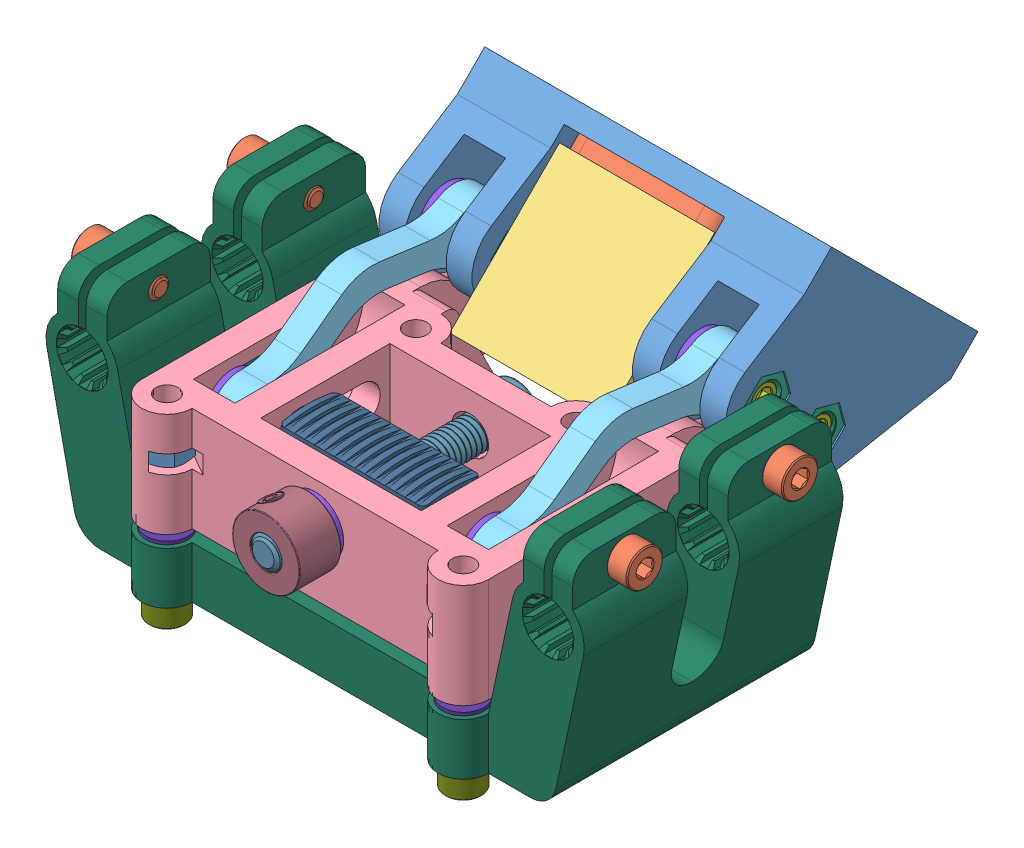
SolidWorks assembly Camera_Angle_Assembly, configuration Default. Lengths in mm.
Overall size (107.85 63.53 108.07).
83 component instances, 20 part files, 71 mates.
Components (placement in the parent):
- Camera_Swing_Bracket-1: Camera_Swing_Bracket [Default] at (-0.7755 -10.5487 -2.6494) x (1 0 0) z (0 -0.707107 0.707107) size (67 43.1 30.6)
- Adapter_Appr-1: Adapter_Appr [Default] at (-30.7755 -11.079 -1.412) x (0 0.707107 0.707107) z (-1 0 0) size (39 2.5 29)
- Camera_Appr-1: Camera_Appr [Default] at (-1.2755 -4.7151 47.3784) x (-1 0 0) z (0 -0.707107 0.707107) size (30 50 30)
- Body_Bracket-2: Body_Bracket [Default] at (-0.7755 -8.7809 23.8671) size (67 20.14 76.95)
- 42-72mm_Linkage_bent_angle-3: 42-72mm_Linkage_bent_angle [Default] at (5.7245 1.8257 34.4737) x (1 0 0) z (0 -0.248282 0.968688) size (5 16.61 54.86)
- 42-72mm_Linkage_bent_angle-4: 42-72mm_Linkage_bent_angle [Default] at (-43.2755 1.8257 34.4737) x (1 0 0) z (0 -0.248282 0.968688) size (5 16.61 54.86)
- Joint_Fastner_Assem-1: Joint_Fastner_Assem [Default] at (21.1511 -8.2693 35.0642) x (0 0.258819 -0.965926) z (0 0.965926 0.258819) size (12.23 18.38 12.23)
  - M6_Shallow_Nuts-1: M6_Shallow_Nuts [90710A038] at (3.1832 5.8266 9.5982) size (10 3.98 11.55)
  - M6_Shallow_Nuts-2: M6_Shallow_Nuts [90710A038] at (3.1832 20.0266 9.5982) size (10 3.98 11.55)
  - Pivot_Bolts-1: Pivot_Bolts [92605A132] at (3.1832 12.6266 9.5982) x (1 0 0) z (0 -1 0) size (6.16 6.24 17.12)
  - Pivot_Washers-1: Pivot_Washers [98689A115] at (3.1832 15.4266 9.5982) x (0.992908 0 0.118882) z (0 1 0) size (11 11 1.5)
  - Pivot_Washers-2: Pivot_Washers [98689A115] at (3.1832 10.4266 9.5982) x (0.997876 0 -0.065141) z (0 -1 0) size (11 11 1.5)
  - Joint_Bushing-1: Joint_Bushing [Default] at (3.1832 10.4266 9.5982) x (0 1 0) z (0 0 1) size (5 7 7)
- Joint_Fastner_Assem-2: Joint_Fastner_Assem [Default] at (21.1511 -14.3398 15.4198) x (0 0.965926 -0.258819) z (0 0.258819 0.965926) size (12.23 18.38 12.23)
  - M6_Shallow_Nuts-1: M6_Shallow_Nuts [90710A038] at (3.1832 5.8266 9.5982) size (10 3.98 11.55)
  - M6_Shallow_Nuts-2: M6_Shallow_Nuts [90710A038] at (3.1832 20.0266 9.5982) size (10 3.98 11.55)
  - Pivot_Bolts-1: Pivot_Bolts [92605A132] at (3.1832 12.6266 9.5982) x (1 0 0) z (0 -1 0) size (6.16 6.24 17.12)
  - Pivot_Washers-1: Pivot_Washers [98689A115] at (3.1832 15.4266 9.5982) x (0.992908 0 0.118882) z (0 1 0) size (11 11 1.5)
  - Pivot_Washers-2: Pivot_Washers [98689A115] at (3.1832 10.4266 9.5982) x (0.997876 0 -0.065141) z (0 -1 0) size (11 11 1.5)
  - Joint_Bushing-1: Joint_Bushing [Default] at (3.1832 10.4266 9.5982) x (0 1 0) z (0 0 1) size (5 7 7)
- Joint_Fastner_Assem-3: Joint_Fastner_Assem [Default] at (-53.7022 0.2569 19.331) x (0 -0.707107 -0.707107) z (0 -0.707107 0.707107) size (12.23 18.38 12.23)
  - M6_Shallow_Nuts-1: M6_Shallow_Nuts [90710A038] at (3.1832 5.8266 9.5982) size (10 3.98 11.55)
  - M6_Shallow_Nuts-2: M6_Shallow_Nuts [90710A038] at (3.1832 20.0266 9.5982) size (10 3.98 11.55)
  - Pivot_Bolts-1: Pivot_Bolts [92605A132] at (3.1832 12.6266 9.5982) x (1 0 0) z (0 -1 0) size (6.16 6.24 17.12)
  - Pivot_Washers-1: Pivot_Washers [98689A115] at (3.1832 15.4266 9.5982) x (0.992908 0 0.118882) z (0 1 0) size (11 11 1.5)
  - Pivot_Washers-2: Pivot_Washers [98689A115] at (3.1832 10.4266 9.5982) x (0.997876 0 -0.065141) z (0 -1 0) size (11 11 1.5)
  - Joint_Bushing-1: Joint_Bushing [Default] at (3.1832 10.4266 9.5982) x (0 1 0) z (0 0 1) size (5 7 7)
- Joint_Fastner_Assem-4: Joint_Fastner_Assem [Default] at (-53.7022 10.8635 29.9376) x (0 -0.707107 -0.707107) z (0 -0.707107 0.707107) size (12.23 18.38 12.23)
  - M6_Shallow_Nuts-1: M6_Shallow_Nuts [90710A038] at (3.1832 5.8266 9.5982) size (10 3.98 11.55)
  - M6_Shallow_Nuts-2: M6_Shallow_Nuts [90710A038] at (3.1832 20.0266 9.5982) size (10 3.98 11.55)
  - Pivot_Bolts-1: Pivot_Bolts [92605A132] at (3.1832 12.6266 9.5982) x (1 0 0) z (0 -1 0) size (6.16 6.24 17.12)
  - Pivot_Washers-1: Pivot_Washers [98689A115] at (3.1832 15.4266 9.5982) x (0.992908 0 0.118882) z (0 1 0) size (11 11 1.5)
  - Pivot_Washers-2: Pivot_Washers [98689A115] at (3.1832 10.4266 9.5982) x (0.997876 0 -0.065141) z (0 -1 0) size (11 11 1.5)
  - Joint_Bushing-1: Joint_Bushing [Default] at (3.1832 10.4266 9.5982) x (0 1 0) z (0 0 1) size (5 7 7)
- Sled_Block-2: Sled_Block [Default] at (-16.2755 -8.7809 70.356) size (28 13.83 11)
- M6_Shallow_Nuts-3: M6_Shallow_Nuts [90710A038] at (-16.2755 -8.7809 79.456) x (0 1 0) z (1 0 0) size (10 3.98 11.55)
- M6_Shallow_Nuts-4: M6_Shallow_Nuts [90710A038] at (-16.2755 -8.7809 72.256) x (0 1 0) z (1 0 0) size (10 3.98 11.55)
- Slider_Bolt_Assembly-1: Slider_Bolt_Assembly [Default] at (2.8001 -20.4339 59.3492) x (1 0 0) z (0 0.5 0.866025) size (22.61 11.45 11.45)
  - Slider-Bolts-1: Slider-Bolts [93070A161] at (-38.5756 1.8384 20.1218) size (22.61 10 10)
  - Slider_Sleeves-1: Slider_Sleeves [Default] at (-34.5756 1.8384 20.1218) x (0 0.999823 0.018793) z (0 -0.018793 0.999823) size (7 11.5 7)
  - Pivot_Washers-1: Pivot_Washers [98689A115] at (-34.5756 1.8384 20.1218) x (0 0 -1) z (1 0 0) size (11 11 1.5)
  - Pivot_Washers-2: Pivot_Washers [98689A115] at (-47.5756 1.8384 20.1218) x (0 0 -1) z (1 0 0) size (11 11 1.5)
  - Pivot_Washers-3: Pivot_Washers [98689A115] at (-39.5756 1.8384 20.1218) x (0 -0.041456 0.99914) z (-1 0 0) size (11 11 1.5)
- Slider_Bolt_Assembly-2: Slider_Bolt_Assembly [Default] at (-35.3512 11.3976 76.9018) x (-1 0 0) z (0 -0.999227 0.039317) size (22.61 11.45 11.45)
  - Slider-Bolts-1: Slider-Bolts [93070A161] at (-38.5756 1.8384 20.1218) size (22.61 10 10)
  - Slider_Sleeves-1: Slider_Sleeves [Default] at (-34.5756 1.8384 20.1218) x (0 0.999823 0.018793) z (0 -0.018793 0.999823) size (7 11.5 7)
  - Pivot_Washers-1: Pivot_Washers [98689A115] at (-34.5756 1.8384 20.1218) x (0 0 -1) z (1 0 0) size (11 11 1.5)
  - Pivot_Washers-2: Pivot_Washers [98689A115] at (-47.5756 1.8384 20.1218) x (0 0 -1) z (1 0 0) size (11 11 1.5)
  - Pivot_Washers-3: Pivot_Washers [98689A115] at (-39.5756 1.8384 20.1218) x (0 -0.041456 0.99914) z (-1 0 0) size (11 11 1.5)
- Pivot_Washers-1: Pivot_Washers [98689A115] at (-16.2755 -8.7809 53.4171) x (0.995184 -0.098022 0) z (0 0 1) size (11 11 1.5)
- Pivot_Washers-2: Pivot_Washers [98689A115] at (-16.2755 -8.7809 86.8671) x (0.604291 0.796764 0) z (0 0 1) size (11 11 1.5)
- Pivot_Washers-3: Pivot_Washers [98689A115] at (-16.2755 -8.7809 88.3671) x (0.569379 0.822075 0) z (0 0 1) size (11 11 1.5)
- Adjuster_Knob_Collar-1: Adjuster_Knob_Collar [57485K66] at (-16.2755 -8.7809 89.8671) x (0.870798 0.491642 0) z (0 0 1) size (13 13 8)
- Lead_Bolt_45mm-1: Lead_Bolt_45mm [91290A204] at (-16.2755 -8.7809 98.4171) size (10 10 49.47)
- Mounting_Plate-2: Mounting_Plate [Default] at (-16.2755 -33.6509 65.8046) x (-1 0 0) z (0 0 -1) size (104 43.39 54.88)
- Spring_Tilt_Bolts_Assembly-1: Spring_Tilt_Bolts_Assembly [Default] at (31.9755 -38.4 78.1988) x (0.999925 0 -0.012246) z (0 1 0) size (8.19 8.19 34.38)
  - M4_30mm_0-7Pitch_Bolt-1: M4_30mm_0-7Pitch_Bolt [91290A180] at (-19.7491 -9.9272 34.1491) size (7 7 34.38)
  - M4_Washer-1: M4_Washer [98689A113] at (-19.7491 -9.9272 14.7491) x (0.999759 0.02194 0) z (0 0 1) size (8 8 0.6)
  - Tilt_Spring-1: Tilt_Spring [94125K379] at (-19.7945 -9.9488 15.6775) x (0.999985 0.000813 -0.005393) z (0.000835 -0.999991 0.004074) size (5.69 18.5 5.69)
  - M4_7mm_0-7Pitch_Nut-1: M4_7mm_0-7Pitch_Nut [90592A090] at (-19.7491 -9.9272 28.9491) x (0.999925 -0.012246 0) z (0.012246 0.999925 0) size (7 3.75 8.08)
  - M4_Washer-2: M4_Washer [98689A113] at (-19.7491 -9.9272 4.1491) x (0.999724 0.023486 0) z (0 0 1) size (8 8 0.6)
- Spring_Tilt_Bolts_Assembly-2: Spring_Tilt_Bolts_Assembly [Default] at (-25.2745 -38.4 78.1988) x (0.999925 0 -0.012246) z (0 1 0) size (8.19 8.19 34.38)
  - M4_30mm_0-7Pitch_Bolt-1: M4_30mm_0-7Pitch_Bolt [91290A180] at (-19.7491 -9.9272 34.1491) size (7 7 34.38)
  - M4_Washer-1: M4_Washer [98689A113] at (-19.7491 -9.9272 14.7491) x (0.999759 0.02194 0) z (0 0 1) size (8 8 0.6)
  - Tilt_Spring-1: Tilt_Spring [94125K379] at (-19.7945 -9.9488 15.6775) x (0.999985 0.000813 -0.005393) z (0.000835 -0.999991 0.004074) size (5.69 18.5 5.69)
  - M4_7mm_0-7Pitch_Nut-1: M4_7mm_0-7Pitch_Nut [90592A090] at (-19.7491 -9.9272 28.9491) x (0.999925 -0.012246 0) z (0.012246 0.999925 0) size (7 3.75 8.08)
  - M4_Washer-2: M4_Washer [98689A113] at (-19.7491 -9.9272 4.1491) x (0.999724 0.023486 0) z (0 0 1) size (8 8 0.6)
- Spring_Tilt_Bolts_Assembly-3: Spring_Tilt_Bolts_Assembly [Default] at (-12.1495 -38.4 43.2488) x (0.999925 0 -0.012246) z (0 1 0) size (8.19 8.19 34.38)
  - M4_30mm_0-7Pitch_Bolt-1: M4_30mm_0-7Pitch_Bolt [91290A180] at (-19.7491 -9.9272 34.1491) size (7 7 34.38)
  - M4_Washer-1: M4_Washer [98689A113] at (-19.7491 -9.9272 14.7491) x (0.999759 0.02194 0) z (0 0 1) size (8 8 0.6)
  - Tilt_Spring-1: Tilt_Spring [94125K379] at (-19.7945 -9.9488 15.6775) x (0.999985 0.000813 -0.005393) z (0.000835 -0.999991 0.004074) size (5.69 18.5 5.69)
  - M4_7mm_0-7Pitch_Nut-1: M4_7mm_0-7Pitch_Nut [90592A090] at (-19.7491 -9.9272 28.9491) x (0.999925 -0.012246 0) z (0.012246 0.999925 0) size (7 3.75 8.08)
  - M4_Washer-2: M4_Washer [98689A113] at (-19.7491 -9.9272 4.1491) x (0.999724 0.023486 0) z (0 0 1) size (8 8 0.6)
- Spring_Tilt_Bolts_Assembly-4: Spring_Tilt_Bolts_Assembly [Default] at (18.8505 -38.4 43.2488) x (0.999925 0 -0.012246) z (0 1 0) size (8.19 8.19 34.38)
  - M4_30mm_0-7Pitch_Bolt-1: M4_30mm_0-7Pitch_Bolt [91290A180] at (-19.7491 -9.9272 34.1491) size (7 7 34.38)
  - M4_Washer-1: M4_Washer [98689A113] at (-19.7491 -9.9272 14.7491) x (0.999759 0.02194 0) z (0 0 1) size (8 8 0.6)
  - Tilt_Spring-1: Tilt_Spring [94125K379] at (-19.7945 -9.9488 15.6775) x (0.999985 0.000813 -0.005393) z (0.000835 -0.999991 0.004074) size (5.69 18.5 5.69)
  - M4_7mm_0-7Pitch_Nut-1: M4_7mm_0-7Pitch_Nut [90592A090] at (-19.7491 -9.9272 28.9491) x (0.999925 -0.012246 0) z (0.012246 0.999925 0) size (7 3.75 8.08)
  - M4_Washer-2: M4_Washer [98689A113] at (-19.7491 -9.9272 4.1491) x (0.999724 0.023486 0) z (0 0 1) size (8 8 0.6)
- M4_10mm_0-7Pitch_Bolt-1: M4_10mm_0-7Pitch_Bolt [91290A144] at (-56.0255 5.7346 48.3671) x (0 0 -1) z (1 0 0) size (7 7 14.32)
- M4_10mm_0-7Pitch_Bolt-2: M4_10mm_0-7Pitch_Bolt [91290A144] at (-56.0255 5.7346 78.3671) x (0 -0.398787 -0.917044) z (1 0 0) size (7 7 14.32)
- M4_10mm_0-7Pitch_Bolt-3: M4_10mm_0-7Pitch_Bolt [91290A144] at (23.4745 5.7346 48.3671) x (0 0 1) z (-1 0 0) size (7 7 14.32)
- M4_10mm_0-7Pitch_Bolt-4: M4_10mm_0-7Pitch_Bolt [91290A144] at (23.4745 5.7346 78.3671) x (0 0 1) z (-1 0 0) size (7 7 14.32)
Mates (geometry in assembly coordinates):
- Concentric1: concentric anti-aligned: circle of Camera_Swing_Bracket-1; circle of Adapter_Appr-1
- Parallel1: parallel aligned: line of Camera_Swing_Bracket-1 through (-31.7755 18.6195 24.751) axis (1 0 0); line of Adapter_Appr-1 through (-27.5755 16.4982 26.1652) axis (1 0 0)
- Coincident1: coincident anti-aligned: plane of Camera_Swing_Bracket-1 through (-16.2755 -9.6648 -3.5333) normal (0 -0.707107 0.707107); plane of Adapter_Appr-1 through (-27.5755 -7.0485 -0.917) normal (0 0.707107 -0.707107)
- Coincident2: coincident anti-aligned: plane of Adapter_Appr-1 through (-27.5755 -8.8163 0.8507) normal (0 -0.707107 0.707107); plane of Camera_Appr-1 through (-1.2755 -11.7861 -2.1191) normal (0 0.707107 -0.707107)
- Coincident5: coincident aligned: plane of Adapter_Appr-1 through (-27.5755 18.2659 24.3974) normal (0 0.707107 0.707107); plane of Camera_Appr-1 through (-1.2755 -4.7151 47.3784) normal (0 0.707107 0.707107)
- Distance3: distance = 1.5 mm anti-aligned: plane of 42-72mm_Linkage_bent_angle-3 through (10.7245 7.273 75.1382) normal (1 0 0); plane of Camera_Swing_Bracket-1 through (12.2245 -10.5487 -2.6494) normal (-1 0 0)
- Concentric4: concentric aligned: circle of Camera_Swing_Bracket-1; circle of 42-72mm_Linkage_bent-1
- Slot2: slot aligned: cylinder of 42-72mm_Linkage_bent_angle-3 through (10.7245 -8.7809 75.856) axis (-1 0 0) radius 3.57; cylinder of Body_Bracket-2 through (17.2245 -8.7809 75.8671) axis (-1 0 0) radius 3.57; cylinder of Body_Bracket-2 through (17.2245 -8.7809 63.8671) axis (-1 0 0) radius 3.57
- Coincident10: coincident aligned: plane of Camera_Swing_Bracket-1 through (17.2245 -8.7809 23.8671) normal (1 0 0); plane of Body_Bracket-2 through (17.2245 -11.2109 46.021) normal (1 0 0)
- Concentric10: concentric anti-aligned: circle of Camera_Swing_Bracket-1; circle of Body_Bracket-1
- Distance4: distance = 0.5 mm anti-aligned: plane of Camera_Appr-1 through (-31.2755 -32.9993 19.0941) normal (-1 0 0); plane of Camera_Swing_Bracket-1 through (-31.7755 -8.7809 23.8671) normal (1 0 0)
- Concentric11: concentric anti-aligned: circle of Camera_Swing_Bracket-1; circle of 42-72mm_Linkage_bent_angle-2
- Distance5: distance = 1.5 mm anti-aligned: plane of 42-72mm_Linkage_bent_angle-4 through (-43.2755 7.273 75.1382) normal (-1 0 0); plane of Body_Bracket-2 through (-44.7755 -2.6734 64.1837) normal (1 0 0)
- Concentric13: concentric aligned: circle of 42-72mm_Linkage_bent_angle-1; circle of 42-72mm_Linkage_bent_angle-2
- Concentric15: concentric aligned: circle of Camera_Swing_Bracket-1; circle of Joint_Fastner_Assem-1/Pivot_Washers-1
- Parallel3: parallel anti-aligned: plane of Camera_Swing_Bracket-1 through (13.7245 6.2871 35.6691) normal (0 -0.707107 -0.707107); plane of Joint_Fastner_Assem-1/M6_Shallow_Nuts-1 through (13.7245 3.32 40.0504) normal (0 0.707107 0.707107)
- Coincident13: coincident anti-aligned: plane of Camera_Swing_Bracket-1 through (13.7245 -10.5487 -2.6494) normal (1 0 0); plane of Joint_Fastner_Assem-1/M6_Shallow_Nuts-1 through (13.7245 -2.2568 38.5562) normal (-1 0 0)
- Concentric16: concentric anti-aligned: circle of Camera_Swing_Bracket-1; circle of Joint_Fastner_Assem-2/M6_Shallow_Nuts-1
- Parallel4: parallel anti-aligned: plane of Camera_Swing_Bracket-1 through (13.7245 -5.5149 20.6011) normal (0 -0.965926 0.258819); plane of Joint_Fastner_Assem-2/M6_Shallow_Nuts-1 through (13.7245 -3.2041 25.3614) normal (0 0.965926 -0.258819)
- Coincident15: coincident anti-aligned: plane of Camera_Swing_Bracket-1 through (13.7245 -10.5487 -2.6494) normal (1 0 0); plane of Joint_Fastner_Assem-2/M6_Shallow_Nuts-1 through (13.7245 -14.3577 22.3728) normal (-1 0 0)
- LimitAngle6: limit planar angle = 0.785398 rad aligned: plane of Body_Bracket-2 through (17.2245 -21.3509 88.3671) normal (0 -1 0); plane of Camera_Appr-1 through (-1.2755 -32.9993 19.0941) normal (0 -0.707107 0.707107)
- Concentric17: concentric aligned: circle of Camera_Swing_Bracket-1; circle of Joint_Fastner_Assem-3/Pivot_Washers-1
- Parallel5: parallel anti-aligned: plane of Camera_Swing_Bracket-1 through (-46.2755 -4.3195 25.0625) normal (0 -0.707107 -0.707107); plane of Joint_Fastner_Assem-3/M6_Shallow_Nuts-1 through (-46.2755 -3.2041 25.3614) normal (0 0.707107 0.707107)
- Coincident16: coincident anti-aligned: plane of Camera_Swing_Bracket-1 through (-46.2755 -10.5487 -2.6494) normal (-1 0 0); plane of Joint_Fastner_Assem-3/M6_Shallow_Nuts-1 through (-46.2755 -3.2041 25.3614) normal (1 0 0)
- Concentric19: concentric anti-aligned: circle of Camera_Swing_Bracket-1; circle of Joint_Fastner_Assem-4/Pivot_Washers-2
- Parallel7: parallel anti-aligned: plane of Camera_Swing_Bracket-1 through (-46.2755 3.0211 38.9351) normal (0 0.258819 -0.965926); plane of Joint_Fastner_Assem-4/M6_Shallow_Nuts-1 through (-46.2755 3.32 40.0504) normal (0 -0.258819 0.965926)
- Coincident18: coincident anti-aligned: plane of Camera_Swing_Bracket-1 through (-46.2755 -10.5487 -2.6494) normal (-1 0 0); plane of Joint_Fastner_Assem-4/M6_Shallow_Nuts-1 through (-46.2755 7.4025 35.968) normal (1 0 0)
- Distance6: distance = 1.5 mm anti-aligned: plane of Sled_Block-2 through (-30.2755 -16.2809 81.356) normal (-1 0 0); plane of Body_Bracket-2 through (-31.7755 -11.2109 46.021) normal (1 0 0)
- Parallel9: parallel aligned: plane of Sled_Block-2 through (-10.502 -8.7809 77.856) normal (-0.866025 -0.5 0); plane of M6_Shallow_Nuts-3 through (-22.049 -8.7809 81.056) normal (-0.866025 -0.5 0)
- Coincident19: coincident anti-aligned: plane of Sled_Block-2 through (-16.2755 -8.7809 77.856) normal (0 0 1); plane of M6_Shallow_Nuts-3 through (-19.1623 -13.7809 77.856) normal (0 0 -1)
- Concentric21: concentric aligned: circle of Sled_Block-1; circle of M6_Shallow_Nuts-3
- Concentric23: concentric aligned: circle of 42-72mm_Linkage_bent_angle-2; circle of Slider_Bolt_Assembly-1/Pivot_Washers-1
- Coincident22: coincident anti-aligned: plane of 42-72mm_Linkage_bent_angle-4 through (-43.2755 7.273 75.1382) normal (-1 0 0); plane of Slider_Bolt_Assembly-1/Pivot_Washers-2 through (-43.2755 -8.7809 75.856) normal (1 0 0)
- Concentric24: concentric anti-aligned: circle of Sled_Block-1; circle of M6_Shallow_Nuts-4
- Coincident23: coincident anti-aligned: plane of Sled_Block-2 through (-16.2755 -8.7809 73.856) normal (0 0 -1); plane of M6_Shallow_Nuts-4 through (-19.1623 -13.7809 73.856) normal (0 0 1)
- Parallel11: parallel anti-aligned: plane of Sled_Block-2 through (-19.1623 -3.7809 73.856) normal (0.866025 -0.5 0); plane of M6_Shallow_Nuts-4 through (-19.1623 -3.7809 73.856) normal (-0.866025 0.5 0)
- Concentric25: concentric anti-aligned: circle of 42-72mm_Linkage_bent_angle-2; circle of Sled_Block-1
- Parallel12: parallel aligned: plane of Body_Bracket-2 through (17.2245 -1.2109 48.3482) normal (0 1 0); plane of Slider_Bolt_Assembly-1/Slider-Bolts-1 through (-45.6555 -10.7809 77.0107) normal (0 1 0)
- Concentric26: concentric anti-aligned: circle of Sled_Block-1; circle of Slider_Bolt_Assembly-2/Pivot_Washers-3
- Coincident24: coincident anti-aligned: plane of 42-72mm_Linkage_bent_angle-3 through (10.7245 7.273 75.1382) normal (1 0 0); plane of Slider_Bolt_Assembly-2/Pivot_Washers-2 through (10.7245 -8.7809 75.856) normal (-1 0 0)
- Coincident26: coincident anti-aligned: plane of Body_Bracket-2 through (-16.2755 -8.7809 54.9171) normal (0 0 -1); plane of Pivot_Washers-1 through (-16.2755 -8.7809 54.9171) normal (0 0 1)
- Concentric29: concentric aligned: circle of Body_Bracket-1; circle of Pivot_Washers-2
- Coincident27: coincident anti-aligned: plane of Body_Bracket-2 through (-16.2755 -8.7809 86.8671) normal (0 0 1); plane of Pivot_Washers-2 through (-16.2755 -8.7809 86.8671) normal (0 0 -1)
- Concentric30: concentric anti-aligned: circle of Body_Bracket-1; circle of Pivot_Washers-1
- Concentric32: concentric aligned: circle of Pivot_Washers-2; circle of Pivot_Washers-3
- Coincident29: coincident anti-aligned: plane of Pivot_Washers-2 through (-16.2755 -8.7809 88.3671) normal (0 0 1); plane of Pivot_Washers-3 through (-16.2755 -8.7809 88.3671) normal (0 0 -1)
- Concentric34: concentric aligned: circle of Pivot_Washers-3; circle of Adjuster_Knob_Collar-1
- Coincident30: coincident anti-aligned: plane of Pivot_Washers-3 through (-16.2755 -8.7809 89.8671) normal (0 0 1); plane of Adjuster_Knob_Collar-1 through (-16.2755 -8.7809 89.8671) normal (0 0 -1)
- Concentric35: concentric anti-aligned: circle of Pivot_Washers-1; circle of Lead_Bolt_45mm-1
- Coincident31: coincident anti-aligned: plane of Pivot_Washers-1 through (-16.2755 -8.7809 53.4171) normal (0 0 -1); circle of Lead_Bolt_45mm-1
- Parallel13: parallel anti-aligned: plane of Body_Bracket-2 through (-32.2198 -16.3509 83.3671) normal (0 0 -1); plane of Sled_Block-2 through (-16.2755 -8.7809 81.356) normal (0 0 1)
- Concentric41: concentric anti-aligned: circle of Body_Bracket-1; circle of Mounting_Plate-1
- Concentric43: concentric anti-aligned: circle of Body_Bracket-1; circle of Mounting_Plate-1
- Concentric44: concentric aligned: circle of Mounting_Plate-1; circle of Spring_Tilt_Bolts_Assembly-1/M4_Washer-1
- Parallel14: parallel anti-aligned: plane of Body_Bracket-2 through (15.8495 -7.8509 90.3878) normal (-0.5 0 -0.866025); plane of Spring_Tilt_Bolts_Assembly-1/M4_7mm_0-7Pitch_Nut-1 through (15.8495 -11.0509 90.3878) normal (0.5 0 0.866025)
- Coincident35: coincident anti-aligned: plane of Body_Bracket-2 through (-0.7755 -7.8509 23.8671) normal (0 -1 0); plane of Spring_Tilt_Bolts_Assembly-1/M4_7mm_0-7Pitch_Nut-1 through (8.8495 -7.8509 90.3878) normal (0 1 0)
- Coincident36: coincident anti-aligned: plane of Mounting_Plate-2 through (-44.9005 -33.6509 88.3671) normal (0 -1 0); plane of Spring_Tilt_Bolts_Assembly-1/M4_Washer-2 through (12.3495 -33.6509 88.3671) normal (0 1 0)
- Concentric45: concentric anti-aligned: circle of Body_Bracket-1; circle of Spring_Tilt_Bolts_Assembly-2/M4_Washer-1
- Coincident37: coincident anti-aligned: plane of Body_Bracket-2 through (-0.7755 -7.8509 23.8671) normal (0 -1 0); plane of Spring_Tilt_Bolts_Assembly-2/M4_7mm_0-7Pitch_Nut-1 through (-48.4005 -7.8509 90.3878) normal (0 1 0)
- Concentric46: concentric anti-aligned: circle of Body_Bracket-1; cylinder of Spring_Tilt_Bolts_Assembly-3/M4_Washer-1 through (-31.7755 -23.0509 53.4171) axis (0 -1 0) radius 4
- Coincident38: coincident anti-aligned: plane of Body_Bracket-2 through (-0.7755 -7.8509 23.8671) normal (0 -1 0); plane of Spring_Tilt_Bolts_Assembly-3/M4_7mm_0-7Pitch_Nut-1 through (-35.2755 -7.8509 55.4378) normal (0 1 0)
- Concentric47: concentric anti-aligned: circle of Body_Bracket-1; circle of Spring_Tilt_Bolts_Assembly-4/M4_Washer-2
- Coincident39: coincident anti-aligned: plane of Body_Bracket-2 through (-0.7755 -7.8509 23.8671) normal (0 -1 0); plane of Spring_Tilt_Bolts_Assembly-4/M4_7mm_0-7Pitch_Nut-1 through (-4.2755 -7.8509 55.4378) normal (0 1 0)
- Concentric53: concentric aligned: circle of Mounting_Plate-1; circle of M4_10mm_0-7Pitch_Bolt-1
- Coincident44: coincident anti-aligned: plane of Mounting_Plate-2 through (-66.0255 1.7346 -8.7981) normal (-1 0 0); plane of M4_10mm_0-7Pitch_Bolt-1 through (-66.0255 5.7346 48.3671) normal (1 0 0)
- Concentric54: concentric aligned: circle of Mounting_Plate-1; circle of M4_10mm_0-7Pitch_Bolt-2
- Coincident45: coincident anti-aligned: plane of Mounting_Plate-2 through (-66.0255 1.7346 -8.7981) normal (-1 0 0); plane of M4_10mm_0-7Pitch_Bolt-2 through (-66.0255 5.7346 78.3671) normal (1 0 0)
- Concentric56: concentric aligned: circle of Mounting_Plate-1; circle of M4_10mm_0-7Pitch_Bolt-3
- Coincident46: coincident anti-aligned: plane of Mounting_Plate-2 through (33.4745 1.7346 -8.7981) normal (1 0 0); plane of M4_10mm_0-7Pitch_Bolt-3 through (33.4745 5.7346 48.3671) normal (-1 0 0)
- Concentric57: concentric aligned: circle of Mounting_Plate-1; circle of M4_10mm_0-7Pitch_Bolt-4
- Coincident47: coincident anti-aligned: plane of Mounting_Plate-2 through (33.4745 1.7346 -8.7981) normal (1 0 0); plane of M4_10mm_0-7Pitch_Bolt-4 through (33.4745 5.7346 78.3671) normal (-1 0 0)
